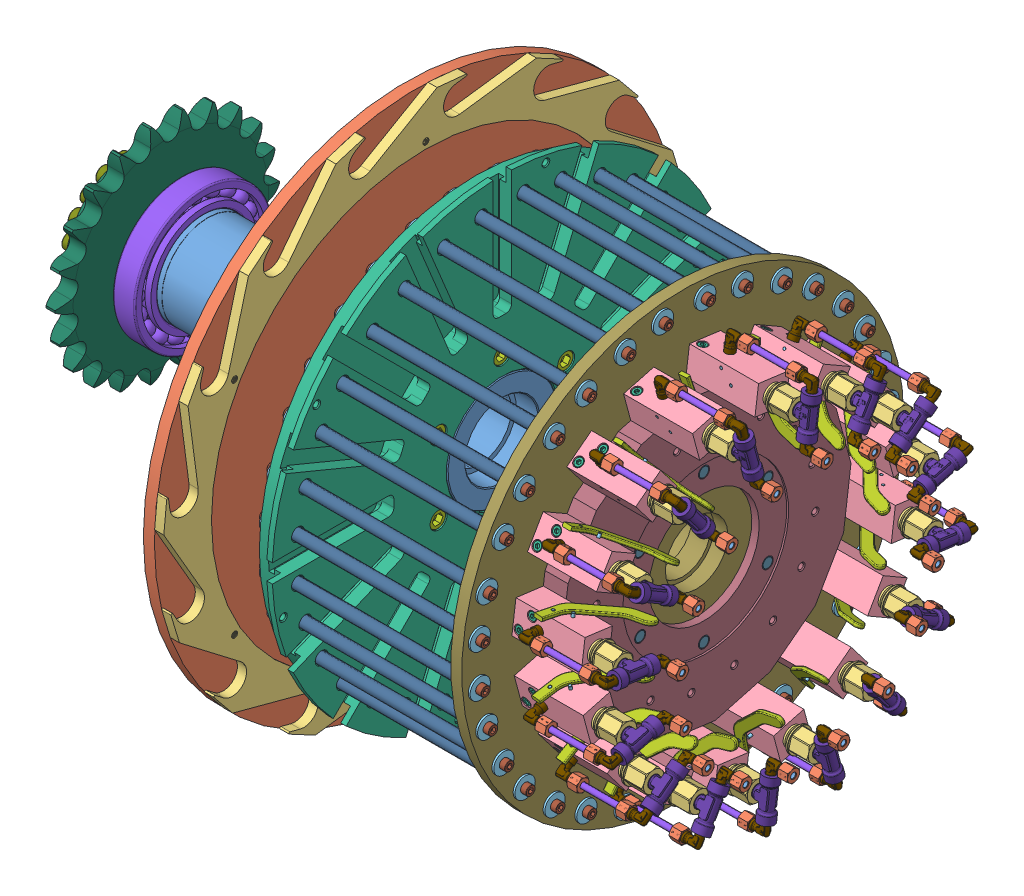
SolidWorks assembly assieme parte rotante, configuration Default. Lengths in mm.
Overall size (749.63 778.63 778.63).
547 component instances, 26 part files, 55 mates.
Components (placement in the parent):
- albero rotazione piatti-1: albero rotazione piatti [Default] at (-23.4119 -16.2033 415) size (415 200 200)
- piatto rotante porta tappi-1: piatto rotante porta tappi [Default] at (15.2184 -16.2033 415) x (0 0 -1) z (1 0 0) size (570 570 20.57)
- disco trasportatore tappi 31-1: disco trasportatore tappi 31 [Default] at (27.2184 -16.2033 415) x (0 -0.5 -0.866025) z (1 0 0) size (570 570 10.42)
- M6 20mm-1: M6 20mm [ISO 4762 M6 x 20 - 20N] at (7.2184 -136.2033 207.1539) x (1 0 0) z (0 -1 0) size (26 10 10)
- rondella m6 22mm-97: rondella m6 22mm [Washer ISO 7094 - 6] at (15.2184 -136.2033 207.1539) x (1 0 0) z (0 0 -1) size (2 22 22)
- rondella m6 22mm-98: rondella m6 22mm [Washer ISO 7094 - 6] at (15.2184 103.7967 207.1539) x (1 0 0) z (0 0.866025 -0.5) size (2 22 22)
- rondella m6 22mm-99: rondella m6 22mm [Washer ISO 7094 - 6] at (15.2184 223.7967 415) x (1 0 0) z (0 0.866025 0.5) size (2 22 22)
- rondella m6 22mm-100: rondella m6 22mm [Washer ISO 7094 - 6] at (15.2184 103.7967 622.8461) size (2 22 22)
- rondella m6 22mm-101: rondella m6 22mm [Washer ISO 7094 - 6] at (15.2184 -136.2033 622.8461) x (1 0 0) z (0 -0.866025 0.5) size (2 22 22)
- rondella m6 22mm-102: rondella m6 22mm [Washer ISO 7094 - 6] at (15.2184 -256.2033 415) x (1 0 0) z (0 -0.866025 -0.5) size (2 22 22)
- M6 20mm-2: M6 20mm [ISO 4762 M6 x 20 - 20N] at (7.2184 103.7967 207.1539) x (1 0 0) z (0 -0.5 -0.866025) size (26 10 10)
- M6 20mm-3: M6 20mm [ISO 4762 M6 x 20 - 20N] at (7.2184 223.7967 415) x (1 0 0) z (0 0.5 -0.866025) size (26 10 10)
- M6 20mm-4: M6 20mm [ISO 4762 M6 x 20 - 20N] at (7.2184 103.7967 622.8461) x (1 0 0) z (0 1 0) size (26 10 10)
- M6 20mm-5: M6 20mm [ISO 4762 M6 x 20 - 20N] at (7.2184 -136.2033 622.8461) x (1 0 0) z (0 0.5 0.866025) size (26 10 10)
- M6 20mm-6: M6 20mm [ISO 4762 M6 x 20 - 20N] at (7.2184 -256.2033 415) x (1 0 0) z (0 -0.5 0.866025) size (26 10 10)
- Disco supporto montaggio e Colonne-1: Disco supporto montaggio e Colonne [Default] at (120.2184 -16.2033 415) x (0 0 -1) z (1 0 0) size (499.6 499.6 29)
- m12 90mm-1: m12 90mm [ISO 4762 M12 x 90 - 90N] at (119.2184 -56.2033 345.718) x (-1 0 0) z (0 -1 0) size (102 18 18)
- m12 90mm-2: m12 90mm [ISO 4762 M12 x 90 - 90N] at (119.2184 -96.2033 415) x (-1 0 0) z (0 -0.5 0.866025) size (102 18 18)
- m12 90mm-3: m12 90mm [ISO 4762 M12 x 90 - 90N] at (119.2184 -56.2033 484.282) x (-1 0 0) z (0 0.5 0.866025) size (102 18 18)
- m12 90mm-4: m12 90mm [ISO 4762 M12 x 90 - 90N] at (119.2184 23.7967 484.282) x (-1 0 0) z (0 1 0) size (102 18 18)
- m12 90mm-5: m12 90mm [ISO 4762 M12 x 90 - 90N] at (119.2184 63.7967 415) x (-1 0 0) z (0 0.5 -0.866025) size (102 18 18)
- m12 90mm-6: m12 90mm [ISO 4762 M12 x 90 - 90N] at (119.2184 23.7967 345.718) x (-1 0 0) z (0 -0.5 -0.866025) size (102 18 18)
- SKF - 6020 - 20,DE,NC,20_68-1: SKF - 6020 - 20,DE,NC,20_68 [SKF - 6020 - 20,DE,NC,20_68] at (-21.7816 -16.2033 415) size (24 150 150)
- SKF - 6020 - 20,DE,NC,20_68-2: SKF - 6020 - 20,DE,NC,20_68 [SKF - 6020 - 20,DE,NC,20_68] at (-216.0316 -16.2033 415) x (1 0 0) z (0 -1 0) size (24 150 150)
- seger 100mm-1: seger 100mm [KS 1336 E - 100] at (-231.0316 -16.2033 415) x (0 0 -1) z (1 0 0) size (107.55 112.98 3)
- asta scorrimento carello-1: asta scorrimento carello [Default] at (203.7184 124.511 241.7588) x (0 0 -1) z (1 0 0) size (12 12 225)
- M6 16mm-7: M6 16mm [ISO 4762 M6 x 16 - 16N] at (83.2184 124.511 241.7588) x (1 0 0) z (0 0 -1) size (22 10 10)
- rondella m6 22mm-1: rondella m6 22mm [Washer ISO 7094 - 6] at (91.2184 124.511 241.7588) x (1 0 0) z (0 0 -1) size (2 22 22)
- M6 16mm-35: M6 16mm [ISO 4762 M6 x 16 - 16N] at (324.2184 124.511 241.7588) x (-1 0 0) z (0 0 1) size (22 10 10)
- rondella m6 22mm-35: rondella m6 22mm [Washer ISO 7094 - 6] at (316.2184 124.511 241.7588) x (-1 0 0) z (0 0 1) size (2 22 22)
- asta scorrimento carello-2: asta scorrimento carello [Default] at (203.7184 157.0379 274.2858) x (0 1 0) z (-1 0 0) size (12 12 225)
- M6 16mm-65: M6 16mm [ISO 4762 M6 x 16 - 16N] at (83.2184 157.0379 274.2858) x (1 0 0) z (0 -1 0) size (22 10 10)
- rondella m6 22mm-65: rondella m6 22mm [Washer ISO 7094 - 6] at (91.2184 157.0379 274.2858) x (1 0 0) z (0 -1 0) size (2 22 22)
- M6 16mm-81: M6 16mm [ISO 4762 M6 x 16 - 16N] at (324.2184 157.0379 274.2858) x (-1 0 0) z (0 1 0) size (22 10 10)
- rondella m6 22mm-81: rondella m6 22mm [Washer ISO 7094 - 6] at (316.2184 157.0379 274.2858) x (-1 0 0) z (0 1 0) size (2 22 22)
- rondella m6 22mm-66: rondella m6 22mm [Washer ISO 7094 - 6] at (91.2184 90.0017 218.7005) x (1 0 0) z (0 -0.92388 0.382683) size (2 22 22)
- rondella m6 22mm-67: rondella m6 22mm [Washer ISO 7094 - 6] at (91.2184 6.7967 193) x (1 0 0) z (0 -0.707107 0.707107) size (2 22 22)
- rondella m6 22mm-68: rondella m6 22mm [Washer ISO 7094 - 6] at (91.2184 -79.9098 201.097) x (1 0 0) z (0 -0.382683 0.92388) size (2 22 22)
- rondella m6 22mm-69: rondella m6 22mm [Washer ISO 7094 - 6] at (91.2184 -156.9175 241.7588) size (2 22 22)
- rondella m6 22mm-70: rondella m6 22mm [Washer ISO 7094 - 6] at (91.2184 -212.5028 308.795) x (1 0 0) z (0 0.382683 0.92388) size (2 22 22)
- rondella m6 22mm-71: rondella m6 22mm [Washer ISO 7094 - 6] at (91.2184 -238.2033 392) x (1 0 0) z (0 0.707107 0.707107) size (2 22 22)
- rondella m6 22mm-72: rondella m6 22mm [Washer ISO 7094 - 6] at (91.2184 -230.1062 478.7065) x (1 0 0) z (0 0.92388 0.382683) size (2 22 22)
- rondella m6 22mm-73: rondella m6 22mm [Washer ISO 7094 - 6] at (91.2184 -189.4444 555.7142) x (1 0 0) z (0 1 0) size (2 22 22)
- rondella m6 22mm-74: rondella m6 22mm [Washer ISO 7094 - 6] at (91.2184 -122.4082 611.2995) x (1 0 0) z (0 0.92388 -0.382683) size (2 22 22)
- rondella m6 22mm-75: rondella m6 22mm [Washer ISO 7094 - 6] at (91.2184 -39.2033 637) x (1 0 0) z (0 0.707107 -0.707107) size (2 22 22)
- rondella m6 22mm-76: rondella m6 22mm [Washer ISO 7094 - 6] at (91.2184 47.5032 628.903) x (1 0 0) z (0 0.382683 -0.92388) size (2 22 22)
- rondella m6 22mm-77: rondella m6 22mm [Washer ISO 7094 - 6] at (91.2184 124.511 588.2412) x (1 0 0) z (0 0 -1) size (2 22 22)
- rondella m6 22mm-78: rondella m6 22mm [Washer ISO 7094 - 6] at (91.2184 180.0963 521.205) x (1 0 0) z (0 -0.382683 -0.92388) size (2 22 22)
- rondella m6 22mm-79: rondella m6 22mm [Washer ISO 7094 - 6] at (91.2184 205.7967 438) x (1 0 0) z (0 -0.707107 -0.707107) size (2 22 22)
- rondella m6 22mm-80: rondella m6 22mm [Washer ISO 7094 - 6] at (91.2184 197.6997 351.2935) x (1 0 0) z (0 -0.92388 -0.382683) size (2 22 22)
- M6 16mm-66: M6 16mm [ISO 4762 M6 x 16 - 16N] at (83.2184 90.0017 218.7005) x (1 0 0) z (0 -0.92388 0.382683) size (22 10 10)
- M6 16mm-67: M6 16mm [ISO 4762 M6 x 16 - 16N] at (83.2184 6.7967 193) x (1 0 0) z (0 -0.707107 0.707107) size (22 10 10)
- M6 16mm-68: M6 16mm [ISO 4762 M6 x 16 - 16N] at (83.2184 -79.9098 201.097) x (1 0 0) z (0 -0.382683 0.92388) size (22 10 10)
- M6 16mm-69: M6 16mm [ISO 4762 M6 x 16 - 16N] at (83.2184 -156.9175 241.7588) size (22 10 10)
- M6 16mm-70: M6 16mm [ISO 4762 M6 x 16 - 16N] at (83.2184 -212.5028 308.795) x (1 0 0) z (0 0.382683 0.92388) size (22 10 10)
- M6 16mm-71: M6 16mm [ISO 4762 M6 x 16 - 16N] at (83.2184 -238.2033 392) x (1 0 0) z (0 0.707107 0.707107) size (22 10 10)
- M6 16mm-72: M6 16mm [ISO 4762 M6 x 16 - 16N] at (83.2184 -230.1062 478.7065) x (1 0 0) z (0 0.92388 0.382683) size (22 10 10)
- M6 16mm-73: M6 16mm [ISO 4762 M6 x 16 - 16N] at (83.2184 -189.4444 555.7142) x (1 0 0) z (0 1 0) size (22 10 10)
- M6 16mm-74: M6 16mm [ISO 4762 M6 x 16 - 16N] at (83.2184 -122.4082 611.2995) x (1 0 0) z (0 0.92388 -0.382683) size (22 10 10)
- M6 16mm-75: M6 16mm [ISO 4762 M6 x 16 - 16N] at (83.2184 -39.2033 637) x (1 0 0) z (0 0.707107 -0.707107) size (22 10 10)
- M6 16mm-76: M6 16mm [ISO 4762 M6 x 16 - 16N] at (83.2184 47.5032 628.903) x (1 0 0) z (0 0.382683 -0.92388) size (22 10 10)
- M6 16mm-77: M6 16mm [ISO 4762 M6 x 16 - 16N] at (83.2184 124.511 588.2412) x (1 0 0) z (0 0 -1) size (22 10 10)
- M6 16mm-78: M6 16mm [ISO 4762 M6 x 16 - 16N] at (83.2184 180.0963 521.205) x (1 0 0) z (0 -0.382683 -0.92388) size (22 10 10)
- M6 16mm-79: M6 16mm [ISO 4762 M6 x 16 - 16N] at (83.2184 205.7967 438) x (1 0 0) z (0 -0.707107 -0.707107) size (22 10 10)
- M6 16mm-80: M6 16mm [ISO 4762 M6 x 16 - 16N] at (83.2184 197.6997 351.2935) x (1 0 0) z (0 -0.92388 -0.382683) size (22 10 10)
- rondella m6 22mm-20: rondella m6 22mm [Washer ISO 7094 - 6] at (91.2184 47.5032 201.097) x (1 0 0) z (0 -0.382683 -0.92388) size (2 22 22)
- rondella m6 22mm-21: rondella m6 22mm [Washer ISO 7094 - 6] at (91.2184 -39.2033 193) x (1 0 0) z (0 -0.707107 -0.707107) size (2 22 22)
- rondella m6 22mm-22: rondella m6 22mm [Washer ISO 7094 - 6] at (91.2184 -122.4082 218.7005) x (1 0 0) z (0 -0.92388 -0.382683) size (2 22 22)
- rondella m6 22mm-23: rondella m6 22mm [Washer ISO 7094 - 6] at (91.2184 -189.4444 274.2858) x (1 0 0) z (0 -1 0) size (2 22 22)
- rondella m6 22mm-24: rondella m6 22mm [Washer ISO 7094 - 6] at (91.2184 -230.1062 351.2935) x (1 0 0) z (0 -0.92388 0.382683) size (2 22 22)
- rondella m6 22mm-25: rondella m6 22mm [Washer ISO 7094 - 6] at (91.2184 -238.2033 438) x (1 0 0) z (0 -0.707107 0.707107) size (2 22 22)
- rondella m6 22mm-26: rondella m6 22mm [Washer ISO 7094 - 6] at (91.2184 -212.5028 521.205) x (1 0 0) z (0 -0.382683 0.92388) size (2 22 22)
- rondella m6 22mm-27: rondella m6 22mm [Washer ISO 7094 - 6] at (91.2184 -156.9175 588.2412) size (2 22 22)
- rondella m6 22mm-28: rondella m6 22mm [Washer ISO 7094 - 6] at (91.2184 -79.9098 628.903) x (1 0 0) z (0 0.382683 0.92388) size (2 22 22)
- rondella m6 22mm-29: rondella m6 22mm [Washer ISO 7094 - 6] at (91.2184 6.7967 637) x (1 0 0) z (0 0.707107 0.707107) size (2 22 22)
- rondella m6 22mm-30: rondella m6 22mm [Washer ISO 7094 - 6] at (91.2184 90.0017 611.2995) x (1 0 0) z (0 0.92388 0.382683) size (2 22 22)
- rondella m6 22mm-31: rondella m6 22mm [Washer ISO 7094 - 6] at (91.2184 157.0379 555.7142) x (1 0 0) z (0 1 0) size (2 22 22)
- rondella m6 22mm-32: rondella m6 22mm [Washer ISO 7094 - 6] at (91.2184 197.6997 478.7065) x (1 0 0) z (0 0.92388 -0.382683) size (2 22 22)
- rondella m6 22mm-33: rondella m6 22mm [Washer ISO 7094 - 6] at (91.2184 205.7967 392) x (1 0 0) z (0 0.707107 -0.707107) size (2 22 22)
- rondella m6 22mm-34: rondella m6 22mm [Washer ISO 7094 - 6] at (91.2184 180.0963 308.795) x (1 0 0) z (0 0.382683 -0.92388) size (2 22 22)
- M6 16mm-20: M6 16mm [ISO 4762 M6 x 16 - 16N] at (83.2184 47.5032 201.097) x (1 0 0) z (0 -0.382683 -0.92388) size (22 10 10)
- M6 16mm-21: M6 16mm [ISO 4762 M6 x 16 - 16N] at (83.2184 -39.2033 193) x (1 0 0) z (0 -0.707107 -0.707107) size (22 10 10)
- M6 16mm-22: M6 16mm [ISO 4762 M6 x 16 - 16N] at (83.2184 -122.4082 218.7005) x (1 0 0) z (0 -0.92388 -0.382683) size (22 10 10)
- M6 16mm-23: M6 16mm [ISO 4762 M6 x 16 - 16N] at (83.2184 -189.4444 274.2858) x (1 0 0) z (0 -1 0) size (22 10 10)
- M6 16mm-24: M6 16mm [ISO 4762 M6 x 16 - 16N] at (83.2184 -230.1062 351.2935) x (1 0 0) z (0 -0.92388 0.382683) size (22 10 10)
- M6 16mm-25: M6 16mm [ISO 4762 M6 x 16 - 16N] at (83.2184 -238.2033 438) x (1 0 0) z (0 -0.707107 0.707107) size (22 10 10)
- M6 16mm-26: M6 16mm [ISO 4762 M6 x 16 - 16N] at (83.2184 -212.5028 521.205) x (1 0 0) z (0 -0.382683 0.92388) size (22 10 10)
- M6 16mm-27: M6 16mm [ISO 4762 M6 x 16 - 16N] at (83.2184 -156.9175 588.2412) size (22 10 10)
- M6 16mm-28: M6 16mm [ISO 4762 M6 x 16 - 16N] at (83.2184 -79.9098 628.903) x (1 0 0) z (0 0.382683 0.92388) size (22 10 10)
- M6 16mm-29: M6 16mm [ISO 4762 M6 x 16 - 16N] at (83.2184 6.7967 637) x (1 0 0) z (0 0.707107 0.707107) size (22 10 10)
- M6 16mm-30: M6 16mm [ISO 4762 M6 x 16 - 16N] at (83.2184 90.0017 611.2995) x (1 0 0) z (0 0.92388 0.382683) size (22 10 10)
- M6 16mm-31: M6 16mm [ISO 4762 M6 x 16 - 16N] at (83.2184 157.0379 555.7142) x (1 0 0) z (0 1 0) size (22 10 10)
- M6 16mm-32: M6 16mm [ISO 4762 M6 x 16 - 16N] at (83.2184 197.6997 478.7065) x (1 0 0) z (0 0.92388 -0.382683) size (22 10 10)
- M6 16mm-33: M6 16mm [ISO 4762 M6 x 16 - 16N] at (83.2184 205.7967 392) x (1 0 0) z (0 0.707107 -0.707107) size (22 10 10)
- M6 16mm-34: M6 16mm [ISO 4762 M6 x 16 - 16N] at (83.2184 180.0963 308.795) x (1 0 0) z (0 0.382683 -0.92388) size (22 10 10)
- M6 16mm-82: M6 16mm [ISO 4762 M6 x 16 - 16N] at (324.2184 90.0017 218.7005) x (-1 0 0) z (0 0.92388 -0.382683) size (22 10 10)
- M6 16mm-83: M6 16mm [ISO 4762 M6 x 16 - 16N] at (324.2184 6.7967 193) x (-1 0 0) z (0 0.707107 -0.707107) size (22 10 10)
- M6 16mm-84: M6 16mm [ISO 4762 M6 x 16 - 16N] at (324.2184 -79.9098 201.097) x (-1 0 0) z (0 0.382683 -0.92388) size (22 10 10)
- M6 16mm-85: M6 16mm [ISO 4762 M6 x 16 - 16N] at (324.2184 -156.9175 241.7588) x (-1 0 0) z (0 0 -1) size (22 10 10)
- M6 16mm-86: M6 16mm [ISO 4762 M6 x 16 - 16N] at (324.2184 -212.5028 308.795) x (-1 0 0) z (0 -0.382683 -0.92388) size (22 10 10)
- M6 16mm-87: M6 16mm [ISO 4762 M6 x 16 - 16N] at (324.2184 -238.2033 392) x (-1 0 0) z (0 -0.707107 -0.707107) size (22 10 10)
- M6 16mm-88: M6 16mm [ISO 4762 M6 x 16 - 16N] at (324.2184 -230.1062 478.7065) x (-1 0 0) z (0 -0.92388 -0.382683) size (22 10 10)
- M6 16mm-89: M6 16mm [ISO 4762 M6 x 16 - 16N] at (324.2184 -189.4444 555.7142) x (-1 0 0) z (0 -1 0) size (22 10 10)
- M6 16mm-90: M6 16mm [ISO 4762 M6 x 16 - 16N] at (324.2184 -122.4082 611.2995) x (-1 0 0) z (0 -0.92388 0.382683) size (22 10 10)
- M6 16mm-91: M6 16mm [ISO 4762 M6 x 16 - 16N] at (324.2184 -39.2033 637) x (-1 0 0) z (0 -0.707107 0.707107) size (22 10 10)
- M6 16mm-92: M6 16mm [ISO 4762 M6 x 16 - 16N] at (324.2184 47.5032 628.903) x (-1 0 0) z (0 -0.382683 0.92388) size (22 10 10)
- M6 16mm-93: M6 16mm [ISO 4762 M6 x 16 - 16N] at (324.2184 124.511 588.2412) x (-1 0 0) z (0 0 1) size (22 10 10)
- M6 16mm-94: M6 16mm [ISO 4762 M6 x 16 - 16N] at (324.2184 180.0963 521.205) x (-1 0 0) z (0 0.382683 0.92388) size (22 10 10)
- M6 16mm-95: M6 16mm [ISO 4762 M6 x 16 - 16N] at (324.2184 205.7967 438) x (-1 0 0) z (0 0.707107 0.707107) size (22 10 10)
- M6 16mm-96: M6 16mm [ISO 4762 M6 x 16 - 16N] at (324.2184 197.6997 351.2935) x (-1 0 0) z (0 0.92388 0.382683) size (22 10 10)
- rondella m6 22mm-82: rondella m6 22mm [Washer ISO 7094 - 6] at (316.2184 90.0017 218.7005) x (-1 0 0) z (0 0.92388 -0.382683) size (2 22 22)
- rondella m6 22mm-83: rondella m6 22mm [Washer ISO 7094 - 6] at (316.2184 6.7967 193) x (-1 0 0) z (0 0.707107 -0.707107) size (2 22 22)
- rondella m6 22mm-84: rondella m6 22mm [Washer ISO 7094 - 6] at (316.2184 -79.9098 201.097) x (-1 0 0) z (0 0.382683 -0.92388) size (2 22 22)
- rondella m6 22mm-85: rondella m6 22mm [Washer ISO 7094 - 6] at (316.2184 -156.9175 241.7588) x (-1 0 0) z (0 0 -1) size (2 22 22)
- rondella m6 22mm-86: rondella m6 22mm [Washer ISO 7094 - 6] at (316.2184 -212.5028 308.795) x (-1 0 0) z (0 -0.382683 -0.92388) size (2 22 22)
- rondella m6 22mm-87: rondella m6 22mm [Washer ISO 7094 - 6] at (316.2184 -238.2033 392) x (-1 0 0) z (0 -0.707107 -0.707107) size (2 22 22)
- rondella m6 22mm-88: rondella m6 22mm [Washer ISO 7094 - 6] at (316.2184 -230.1062 478.7065) x (-1 0 0) z (0 -0.92388 -0.382683) size (2 22 22)
- rondella m6 22mm-89: rondella m6 22mm [Washer ISO 7094 - 6] at (316.2184 -189.4444 555.7142) x (-1 0 0) z (0 -1 0) size (2 22 22)
- rondella m6 22mm-90: rondella m6 22mm [Washer ISO 7094 - 6] at (316.2184 -122.4082 611.2995) x (-1 0 0) z (0 -0.92388 0.382683) size (2 22 22)
- rondella m6 22mm-91: rondella m6 22mm [Washer ISO 7094 - 6] at (316.2184 -39.2033 637) x (-1 0 0) z (0 -0.707107 0.707107) size (2 22 22)
- rondella m6 22mm-92: rondella m6 22mm [Washer ISO 7094 - 6] at (316.2184 47.5032 628.903) x (-1 0 0) z (0 -0.382683 0.92388) size (2 22 22)
- rondella m6 22mm-93: rondella m6 22mm [Washer ISO 7094 - 6] at (316.2184 124.511 588.2412) x (-1 0 0) z (0 0 1) size (2 22 22)
- rondella m6 22mm-94: rondella m6 22mm [Washer ISO 7094 - 6] at (316.2184 180.0963 521.205) x (-1 0 0) z (0 0.382683 0.92388) size (2 22 22)
- rondella m6 22mm-95: rondella m6 22mm [Washer ISO 7094 - 6] at (316.2184 205.7967 438) x (-1 0 0) z (0 0.707107 0.707107) size (2 22 22)
- rondella m6 22mm-96: rondella m6 22mm [Washer ISO 7094 - 6] at (316.2184 197.6997 351.2935) x (-1 0 0) z (0 0.92388 0.382683) size (2 22 22)
- M6 16mm-50: M6 16mm [ISO 4762 M6 x 16 - 16N] at (324.2184 47.5032 201.097) x (-1 0 0) z (0 0.382683 0.92388) size (22 10 10)
- M6 16mm-51: M6 16mm [ISO 4762 M6 x 16 - 16N] at (324.2184 -39.2033 193) x (-1 0 0) z (0 0.707107 0.707107) size (22 10 10)
- M6 16mm-52: M6 16mm [ISO 4762 M6 x 16 - 16N] at (324.2184 -122.4082 218.7005) x (-1 0 0) z (0 0.92388 0.382683) size (22 10 10)
- M6 16mm-53: M6 16mm [ISO 4762 M6 x 16 - 16N] at (324.2184 -189.4444 274.2858) x (-1 0 0) z (0 1 0) size (22 10 10)
- M6 16mm-54: M6 16mm [ISO 4762 M6 x 16 - 16N] at (324.2184 -230.1062 351.2935) x (-1 0 0) z (0 0.92388 -0.382683) size (22 10 10)
- M6 16mm-55: M6 16mm [ISO 4762 M6 x 16 - 16N] at (324.2184 -238.2033 438) x (-1 0 0) z (0 0.707107 -0.707107) size (22 10 10)
- M6 16mm-56: M6 16mm [ISO 4762 M6 x 16 - 16N] at (324.2184 -212.5028 521.205) x (-1 0 0) z (0 0.382683 -0.92388) size (22 10 10)
- M6 16mm-57: M6 16mm [ISO 4762 M6 x 16 - 16N] at (324.2184 -156.9175 588.2412) x (-1 0 0) z (0 0 -1) size (22 10 10)
- M6 16mm-58: M6 16mm [ISO 4762 M6 x 16 - 16N] at (324.2184 -79.9098 628.903) x (-1 0 0) z (0 -0.382683 -0.92388) size (22 10 10)
- M6 16mm-59: M6 16mm [ISO 4762 M6 x 16 - 16N] at (324.2184 6.7967 637) x (-1 0 0) z (0 -0.707107 -0.707107) size (22 10 10)
- M6 16mm-60: M6 16mm [ISO 4762 M6 x 16 - 16N] at (324.2184 90.0017 611.2995) x (-1 0 0) z (0 -0.92388 -0.382683) size (22 10 10)
- M6 16mm-61: M6 16mm [ISO 4762 M6 x 16 - 16N] at (324.2184 157.0379 555.7142) x (-1 0 0) z (0 -1 0) size (22 10 10)
- M6 16mm-62: M6 16mm [ISO 4762 M6 x 16 - 16N] at (324.2184 197.6997 478.7065) x (-1 0 0) z (0 -0.92388 0.382683) size (22 10 10)
- M6 16mm-63: M6 16mm [ISO 4762 M6 x 16 - 16N] at (324.2184 205.7967 392) x (-1 0 0) z (0 -0.707107 0.707107) size (22 10 10)
- M6 16mm-64: M6 16mm [ISO 4762 M6 x 16 - 16N] at (324.2184 180.0963 308.795) x (-1 0 0) z (0 -0.382683 0.92388) size (22 10 10)
- rondella m6 22mm-50: rondella m6 22mm [Washer ISO 7094 - 6] at (316.2184 47.5032 201.097) x (-1 0 0) z (0 0.382683 0.92388) size (2 22 22)
- rondella m6 22mm-51: rondella m6 22mm [Washer ISO 7094 - 6] at (316.2184 -39.2033 193) x (-1 0 0) z (0 0.707107 0.707107) size (2 22 22)
- rondella m6 22mm-52: rondella m6 22mm [Washer ISO 7094 - 6] at (316.2184 -122.4082 218.7005) x (-1 0 0) z (0 0.92388 0.382683) size (2 22 22)
- rondella m6 22mm-53: rondella m6 22mm [Washer ISO 7094 - 6] at (316.2184 -189.4444 274.2858) x (-1 0 0) z (0 1 0) size (2 22 22)
- rondella m6 22mm-54: rondella m6 22mm [Washer ISO 7094 - 6] at (316.2184 -230.1062 351.2935) x (-1 0 0) z (0 0.92388 -0.382683) size (2 22 22)
- rondella m6 22mm-55: rondella m6 22mm [Washer ISO 7094 - 6] at (316.2184 -238.2033 438) x (-1 0 0) z (0 0.707107 -0.707107) size (2 22 22)
- rondella m6 22mm-56: rondella m6 22mm [Washer ISO 7094 - 6] at (316.2184 -212.5028 521.205) x (-1 0 0) z (0 0.382683 -0.92388) size (2 22 22)
- rondella m6 22mm-57: rondella m6 22mm [Washer ISO 7094 - 6] at (316.2184 -156.9175 588.2412) x (-1 0 0) z (0 0 -1) size (2 22 22)
- rondella m6 22mm-58: rondella m6 22mm [Washer ISO 7094 - 6] at (316.2184 -79.9098 628.903) x (-1 0 0) z (0 -0.382683 -0.92388) size (2 22 22)
- rondella m6 22mm-59: rondella m6 22mm [Washer ISO 7094 - 6] at (316.2184 6.7967 637) x (-1 0 0) z (0 -0.707107 -0.707107) size (2 22 22)
- rondella m6 22mm-60: rondella m6 22mm [Washer ISO 7094 - 6] at (316.2184 90.0017 611.2995) x (-1 0 0) z (0 -0.92388 -0.382683) size (2 22 22)
- rondella m6 22mm-61: rondella m6 22mm [Washer ISO 7094 - 6] at (316.2184 157.0379 555.7142) x (-1 0 0) z (0 -1 0) size (2 22 22)
- rondella m6 22mm-62: rondella m6 22mm [Washer ISO 7094 - 6] at (316.2184 197.6997 478.7065) x (-1 0 0) z (0 -0.92388 0.382683) size (2 22 22)
- rondella m6 22mm-63: rondella m6 22mm [Washer ISO 7094 - 6] at (316.2184 205.7967 392) x (-1 0 0) z (0 -0.707107 0.707107) size (2 22 22)
- rondella m6 22mm-64: rondella m6 22mm [Washer ISO 7094 - 6] at (316.2184 180.0963 308.795) x (-1 0 0) z (0 -0.382683 0.92388) size (2 22 22)
- asta scorrimento carello-3: asta scorrimento carello [Default] at (203.7184 47.5032 201.097) x (0 -0.382683 -0.92388) z (1 0 0) size (12 12 225)
- asta scorrimento carello-4: asta scorrimento carello [Default] at (203.7184 -39.2033 193) x (0 -0.707107 -0.707107) z (1 0 0) size (12 12 225)
- asta scorrimento carello-5: asta scorrimento carello [Default] at (203.7184 -122.4082 218.7005) x (0 -0.92388 -0.382683) z (1 0 0) size (12 12 225)
- asta scorrimento carello-6: asta scorrimento carello [Default] at (203.7184 -189.4444 274.2858) x (0 -1 0) z (1 0 0) size (12 12 225)
- asta scorrimento carello-7: asta scorrimento carello [Default] at (203.7184 -230.1062 351.2935) x (0 -0.92388 0.382683) z (1 0 0) size (12 12 225)
- asta scorrimento carello-8: asta scorrimento carello [Default] at (203.7184 -238.2033 438) x (0 -0.707107 0.707107) z (1 0 0) size (12 12 225)
- asta scorrimento carello-9: asta scorrimento carello [Default] at (203.7184 -212.5028 521.205) x (0 -0.382683 0.92388) z (1 0 0) size (12 12 225)
- asta scorrimento carello-10: asta scorrimento carello [Default] at (203.7184 -156.9175 588.2412) x (0 0 1) z (1 0 0) size (12 12 225)
- asta scorrimento carello-11: asta scorrimento carello [Default] at (203.7184 -79.9098 628.903) x (0 0.382683 0.92388) z (1 0 0) size (12 12 225)
- asta scorrimento carello-12: asta scorrimento carello [Default] at (203.7184 6.7967 637) x (0 0.707107 0.707107) z (1 0 0) size (12 12 225)
- asta scorrimento carello-13: asta scorrimento carello [Default] at (203.7184 90.0017 611.2995) x (0 0.92388 0.382683) z (1 0 0) size (12 12 225)
- asta scorrimento carello-14: asta scorrimento carello [Default] at (203.7184 157.0379 555.7142) x (0 1 0) z (1 0 0) size (12 12 225)
- asta scorrimento carello-15: asta scorrimento carello [Default] at (203.7184 197.6997 478.7065) x (0 0.92388 -0.382683) z (1 0 0) size (12 12 225)
- asta scorrimento carello-16: asta scorrimento carello [Default] at (203.7184 205.7967 392) x (0 0.707107 -0.707107) z (1 0 0) size (12 12 225)
- asta scorrimento carello-17: asta scorrimento carello [Default] at (203.7184 180.0963 308.795) x (0 0.382683 -0.92388) z (1 0 0) size (12 12 225)
- asta scorrimento carello-18: asta scorrimento carello [Default] at (203.7184 90.0017 218.7005) x (0 0.92388 -0.382683) z (-1 0 0) size (12 12 225)
- asta scorrimento carello-19: asta scorrimento carello [Default] at (203.7184 6.7967 193) x (0 0.707107 -0.707107) z (-1 0 0) size (12 12 225)
- asta scorrimento carello-20: asta scorrimento carello [Default] at (203.7184 -79.9098 201.097) x (0 0.382683 -0.92388) z (-1 0 0) size (12 12 225)
- asta scorrimento carello-21: asta scorrimento carello [Default] at (203.7184 -156.9175 241.7588) x (0 0 -1) z (-1 0 0) size (12 12 225)
- asta scorrimento carello-22: asta scorrimento carello [Default] at (203.7184 -212.5028 308.795) x (0 -0.382683 -0.92388) z (-1 0 0) size (12 12 225)
- asta scorrimento carello-23: asta scorrimento carello [Default] at (203.7184 -238.2033 392) x (0 -0.707107 -0.707107) z (-1 0 0) size (12 12 225)
- asta scorrimento carello-24: asta scorrimento carello [Default] at (203.7184 -230.1062 478.7065) x (0 -0.92388 -0.382683) z (-1 0 0) size (12 12 225)
- asta scorrimento carello-25: asta scorrimento carello [Default] at (203.7184 -189.4444 555.7142) x (0 -1 0) z (-1 0 0) size (12 12 225)
- asta scorrimento carello-26: asta scorrimento carello [Default] at (203.7184 -122.4082 611.2995) x (0 -0.92388 0.382683) z (-1 0 0) size (12 12 225)
- asta scorrimento carello-27: asta scorrimento carello [Default] at (203.7184 -39.2033 637) x (0 -0.707107 0.707107) z (-1 0 0) size (12 12 225)
- asta scorrimento carello-28: asta scorrimento carello [Default] at (203.7184 47.5032 628.903) x (0 -0.382683 0.92388) z (-1 0 0) size (12 12 225)
- asta scorrimento carello-29: asta scorrimento carello [Default] at (203.7184 124.511 588.2412) x (0 0 1) z (-1 0 0) size (12 12 225)
- asta scorrimento carello-30: asta scorrimento carello [Default] at (203.7184 180.0963 521.205) x (0 0.382683 0.92388) z (-1 0 0) size (12 12 225)
- asta scorrimento carello-31: asta scorrimento carello [Default] at (203.7184 205.7967 438) x (0 0.707107 0.707107) z (-1 0 0) size (12 12 225)
- asta scorrimento carello-32: asta scorrimento carello [Default] at (203.7184 197.6997 351.2935) x (0 0.92388 0.382683) z (-1 0 0) size (12 12 225)
- disco trascinato porta distributore vuoto-2: disco trascinato porta distributore vuoto [Default] at (316.2184 -16.2033 415) x (0 0 1) z (-1 0 0) size (480 480 50)
- Distributore Rotante-1: Distributore Rotante [Default] at (341.2184 -16.2033 415) x (0 -0.5 -0.866025) z (1 0 0) size (310 310 25.54)
- m12 35mm-97: m12 35mm [ISO 4762 M12 x 35 - 35N] at (292.2184 -96.2033 415) size (47 18 18)
- m12 35mm-98: m12 35mm [ISO 4762 M12 x 35 - 35N] at (292.2184 -56.2033 484.282) x (1 0 0) z (0 0.866025 0.5) size (47 18 18)
- m12 35mm-99: m12 35mm [ISO 4762 M12 x 35 - 35N] at (292.2184 23.7967 484.282) x (1 0 0) z (0 0.866025 -0.5) size (47 18 18)
- m12 35mm-100: m12 35mm [ISO 4762 M12 x 35 - 35N] at (292.2184 63.7967 415) x (1 0 0) z (0 0 -1) size (47 18 18)
- m12 35mm-101: m12 35mm [ISO 4762 M12 x 35 - 35N] at (292.2184 23.7967 345.718) x (1 0 0) z (0 -0.866025 -0.5) size (47 18 18)
- m12 35mm-102: m12 35mm [ISO 4762 M12 x 35 - 35N] at (292.2184 -56.2033 345.718) x (1 0 0) z (0 -0.866025 0.5) size (47 18 18)
- pulegia z =50-3: pulegia z =50 [Chain wheel ISO - 22Z 20A-1 --22SB150H40L95.0N] at (-257.7416 -16.2033 415) size (41.88 241.57 243.73)
- calettatore d95-1: calettatore d95 [Default] at (-268.7821 -16.2033 415) size (39.5 135 135)
- AssiemeValvola-1: AssiemeValvola [Default] at (431.5008 -101.2033 267.7757) x (0 0.5 0.866025) z (0 0.866025 -0.5) size (90.26 138.63 38)
  - RaccordoT-1: RaccordoT [Default] at origin size (43 29.75 16.5)
  - Raccordo a L-1: Raccordo a L [Default] at (-30 0 0) x (0 -1 0) z (0 0 -1) size (28.34 25.51 14.01)
    - 1809_06_10_01-1: 1809_06_10_01 [Default] at origin size (22.49 23 10)
    - 1809_06_10_02-1: 1809_06_10_02 [Default] at origin size (6.5 8.5 8.5)
    - 1809_06_10_03-1: 1809_06_10_03 [Default] at origin size (11.02 15.01 14.01)
  - Raccordo a L-2: Raccordo a L [Default] at (30 0 0) x (0 1 0) z (0 0 -1) size (28.34 25.51 14.01)
    - 1809_06_10_01-1: 1809_06_10_01 [Default] at origin size (22.49 23 10)
    - 1809_06_10_02-1: 1809_06_10_02 [Default] at origin size (6.5 8.5 8.5)
    - 1809_06_10_03-1: 1809_06_10_03 [Default] at origin size (11.02 15.01 14.01)
  - TappoChiusura-1: TappoChiusura [Default] at (0 -32 0) x (0 -1 0) z (0 0 1) size (38.28 26.74 26.74)
  - CorpoValvola-1: CorpoValvola [Default] at (-15 -115.2824 0) size (30 75 34)
  - Raccordo a L-3: Raccordo a L [Default] at (-30 -88.2824 0) x (0 1 0) z (0 0 1) size (28.34 25.51 14.01)
    - 1809_06_10_01-1: 1809_06_10_01 [Default] at origin size (22.49 23 10)
    - 1809_06_10_02-1: 1809_06_10_02 [Default] at origin size (6.5 8.5 8.5)
    - 1809_06_10_03-1: 1809_06_10_03 [Default] at origin size (11.02 15.01 14.01)
  - Spina_3x38-1: Spina_3x38 [Default] at (0 -68.2824 -21) x (-1 0 0) z (0 0 1) size (3 3 38)
  - Spina_3x38-2: Spina_3x38 [Default] at (-10 -80.2824 -21) x (0.996193 0.087174 0) z (0 0 1) size (3 3 38)
  - M5 40mm-3: M5 40mm [ISO 4762 M5 x 40 - 40N] at (-14.6 -108.7824 9) size (45 8.5 8.5)
  - M5 40mm-2: M5 40mm [ISO 4762 M5 x 40 - 40N] at (-14.6 -96.7824 -9) size (45 8.5 8.5)
  - LevaValvola-1: LevaValvola [Default] at (-24.507 -86.571 -17) x (0.996193 0.087174 0) z (0 0 1) size (77.55 60.2 4)
  - Tubo-1: Tubo [Default] at (-30 -15.9665 0) x (1 0 0) z (0 -1 0) size (6 6 56.4)
- AssiemeValvola-2: AssiemeValvola [Default] at (431.5008 -151.0733 311.5106) x (0 0.793353 0.608761) z (0 0.608761 -0.793353) size (90.26 138.63 38)
  - RaccordoT-1: RaccordoT [Default] at origin size (43 29.75 16.5)
  - Raccordo a L-1: Raccordo a L [Default] at (-30 0 0) x (0 -1 0) z (0 0 -1) size (28.34 25.51 14.01)
    - 1809_06_10_01-1: 1809_06_10_01 [Default] at origin size (22.49 23 10)
    - 1809_06_10_02-1: 1809_06_10_02 [Default] at origin size (6.5 8.5 8.5)
    - 1809_06_10_03-1: 1809_06_10_03 [Default] at origin size (11.02 15.01 14.01)
  - Raccordo a L-2: Raccordo a L [Default] at (30 0 0) x (0 1 0) z (0 0 -1) size (28.34 25.51 14.01)
    - 1809_06_10_01-1: 1809_06_10_01 [Default] at origin size (22.49 23 10)
    - 1809_06_10_02-1: 1809_06_10_02 [Default] at origin size (6.5 8.5 8.5)
    - 1809_06_10_03-1: 1809_06_10_03 [Default] at origin size (11.02 15.01 14.01)
  - TappoChiusura-1: TappoChiusura [Default] at (0 -32 0) x (0 -1 0) z (0 0 1) size (38.28 26.74 26.74)
  - CorpoValvola-1: CorpoValvola [Default] at (-15 -115.2824 0) size (30 75 34)
  - Raccordo a L-3: Raccordo a L [Default] at (-30 -88.2824 0) x (0 1 0) z (0 0 1) size (28.34 25.51 14.01)
    - 1809_06_10_01-1: 1809_06_10_01 [Default] at origin size (22.49 23 10)
    - 1809_06_10_02-1: 1809_06_10_02 [Default] at origin size (6.5 8.5 8.5)
    - 1809_06_10_03-1: 1809_06_10_03 [Default] at origin size (11.02 15.01 14.01)
  - Spina_3x38-1: Spina_3x38 [Default] at (0 -68.2824 -21) x (-1 0 0) z (0 0 1) size (3 3 38)
  - Spina_3x38-2: Spina_3x38 [Default] at (-10 -80.2824 -21) x (0.996193 0.087174 0) z (0 0 1) size (3 3 38)
  - M5 40mm-3: M5 40mm [ISO 4762 M5 x 40 - 40N] at (-14.6 -108.7824 9) size (45 8.5 8.5)
  - M5 40mm-2: M5 40mm [ISO 4762 M5 x 40 - 40N] at (-14.6 -96.7824 -9) size (45 8.5 8.5)
  - LevaValvola-1: LevaValvola [Default] at (-24.507 -86.571 -17) x (0.996193 0.087174 0) z (0 0 1) size (77.55 60.2 4)
  - Tubo-1: Tubo [Default] at (-30 -15.9665 0) x (1 0 0) z (0 -1 0) size (6 6 56.4)
- AssiemeValvola-3: AssiemeValvola [Default] at (431.5008 -180.4107 371.0008) x (0 0.965926 0.258819) z (0 0.258819 -0.965926) size (90.26 138.63 38)
  - RaccordoT-1: RaccordoT [Default] at origin size (43 29.75 16.5)
  - Raccordo a L-1: Raccordo a L [Default] at (-30 0 0) x (0 -1 0) z (0 0 -1) size (28.34 25.51 14.01)
    - 1809_06_10_01-1: 1809_06_10_01 [Default] at origin size (22.49 23 10)
    - 1809_06_10_02-1: 1809_06_10_02 [Default] at origin size (6.5 8.5 8.5)
    - 1809_06_10_03-1: 1809_06_10_03 [Default] at origin size (11.02 15.01 14.01)
  - Raccordo a L-2: Raccordo a L [Default] at (30 0 0) x (0 1 0) z (0 0 -1) size (28.34 25.51 14.01)
    - 1809_06_10_01-1: 1809_06_10_01 [Default] at origin size (22.49 23 10)
    - 1809_06_10_02-1: 1809_06_10_02 [Default] at origin size (6.5 8.5 8.5)
    - 1809_06_10_03-1: 1809_06_10_03 [Default] at origin size (11.02 15.01 14.01)
  - TappoChiusura-1: TappoChiusura [Default] at (0 -32 0) x (0 -1 0) z (0 0 1) size (38.28 26.74 26.74)
  - CorpoValvola-1: CorpoValvola [Default] at (-15 -115.2824 0) size (30 75 34)
  - Raccordo a L-3: Raccordo a L [Default] at (-30 -88.2824 0) x (0 1 0) z (0 0 1) size (28.34 25.51 14.01)
    - 1809_06_10_01-1: 1809_06_10_01 [Default] at origin size (22.49 23 10)
    - 1809_06_10_02-1: 1809_06_10_02 [Default] at origin size (6.5 8.5 8.5)
    - 1809_06_10_03-1: 1809_06_10_03 [Default] at origin size (11.02 15.01 14.01)
  - Spina_3x38-1: Spina_3x38 [Default] at (0 -68.2824 -21) x (-1 0 0) z (0 0 1) size (3 3 38)
  - Spina_3x38-2: Spina_3x38 [Default] at (-10 -80.2824 -21) x (0.996193 0.087174 0) z (0 0 1) size (3 3 38)
  - M5 40mm-3: M5 40mm [ISO 4762 M5 x 40 - 40N] at (-14.6 -108.7824 9) size (45 8.5 8.5)
  - M5 40mm-2: M5 40mm [ISO 4762 M5 x 40 - 40N] at (-14.6 -96.7824 -9) size (45 8.5 8.5)
  - LevaValvola-1: LevaValvola [Default] at (-24.507 -86.571 -17) x (0.996193 0.087174 0) z (0 0 1) size (77.55 60.2 4)
  - Tubo-1: Tubo [Default] at (-30 -15.9665 0) x (1 0 0) z (0 -1 0) size (6 6 56.4)
- AssiemeValvola-4: AssiemeValvola [Default] at (431.5008 -184.7489 437.1895) x (0 0.991445 -0.130526) z (0 -0.130526 -0.991445) size (90.26 138.63 38)
  - RaccordoT-1: RaccordoT [Default] at origin size (43 29.75 16.5)
  - Raccordo a L-1: Raccordo a L [Default] at (-30 0 0) x (0 -1 0) z (0 0 -1) size (28.34 25.51 14.01)
    - 1809_06_10_01-1: 1809_06_10_01 [Default] at origin size (22.49 23 10)
    - 1809_06_10_02-1: 1809_06_10_02 [Default] at origin size (6.5 8.5 8.5)
    - 1809_06_10_03-1: 1809_06_10_03 [Default] at origin size (11.02 15.01 14.01)
  - Raccordo a L-2: Raccordo a L [Default] at (30 0 0) x (0 1 0) z (0 0 -1) size (28.34 25.51 14.01)
    - 1809_06_10_01-1: 1809_06_10_01 [Default] at origin size (22.49 23 10)
    - 1809_06_10_02-1: 1809_06_10_02 [Default] at origin size (6.5 8.5 8.5)
    - 1809_06_10_03-1: 1809_06_10_03 [Default] at origin size (11.02 15.01 14.01)
  - TappoChiusura-1: TappoChiusura [Default] at (0 -32 0) x (0 -1 0) z (0 0 1) size (38.28 26.74 26.74)
  - CorpoValvola-1: CorpoValvola [Default] at (-15 -115.2824 0) size (30 75 34)
  - Raccordo a L-3: Raccordo a L [Default] at (-30 -88.2824 0) x (0 1 0) z (0 0 1) size (28.34 25.51 14.01)
    - 1809_06_10_01-1: 1809_06_10_01 [Default] at origin size (22.49 23 10)
    - 1809_06_10_02-1: 1809_06_10_02 [Default] at origin size (6.5 8.5 8.5)
    - 1809_06_10_03-1: 1809_06_10_03 [Default] at origin size (11.02 15.01 14.01)
  - Spina_3x38-1: Spina_3x38 [Default] at (0 -68.2824 -21) x (-1 0 0) z (0 0 1) size (3 3 38)
  - Spina_3x38-2: Spina_3x38 [Default] at (-10 -80.2824 -21) x (0.996193 0.087174 0) z (0 0 1) size (3 3 38)
  - M5 40mm-3: M5 40mm [ISO 4762 M5 x 40 - 40N] at (-14.6 -108.7824 9) size (45 8.5 8.5)
  - M5 40mm-2: M5 40mm [ISO 4762 M5 x 40 - 40N] at (-14.6 -96.7824 -9) size (45 8.5 8.5)
  - LevaValvola-1: LevaValvola [Default] at (-24.507 -86.571 -17) x (0.996193 0.087174 0) z (0 0 1) size (77.55 60.2 4)
  - Tubo-1: Tubo [Default] at (-30 -15.9665 0) x (1 0 0) z (0 -1 0) size (6 6 56.4)
- AssiemeValvola-5: AssiemeValvola [Default] at (431.5008 -163.4276 500) x (0 0.866025 -0.5) z (0 -0.5 -0.866025) size (90.26 138.63 38)
  - RaccordoT-1: RaccordoT [Default] at origin size (43 29.75 16.5)
  - Raccordo a L-1: Raccordo a L [Default] at (-30 0 0) x (0 -1 0) z (0 0 -1) size (28.34 25.51 14.01)
    - 1809_06_10_01-1: 1809_06_10_01 [Default] at origin size (22.49 23 10)
    - 1809_06_10_02-1: 1809_06_10_02 [Default] at origin size (6.5 8.5 8.5)
    - 1809_06_10_03-1: 1809_06_10_03 [Default] at origin size (11.02 15.01 14.01)
  - Raccordo a L-2: Raccordo a L [Default] at (30 0 0) x (0 1 0) z (0 0 -1) size (28.34 25.51 14.01)
    - 1809_06_10_01-1: 1809_06_10_01 [Default] at origin size (22.49 23 10)
    - 1809_06_10_02-1: 1809_06_10_02 [Default] at origin size (6.5 8.5 8.5)
    - 1809_06_10_03-1: 1809_06_10_03 [Default] at origin size (11.02 15.01 14.01)
  - TappoChiusura-1: TappoChiusura [Default] at (0 -32 0) x (0 -1 0) z (0 0 1) size (38.28 26.74 26.74)
  - CorpoValvola-1: CorpoValvola [Default] at (-15 -115.2824 0) size (30 75 34)
  - Raccordo a L-3: Raccordo a L [Default] at (-30 -88.2824 0) x (0 1 0) z (0 0 1) size (28.34 25.51 14.01)
    - 1809_06_10_01-1: 1809_06_10_01 [Default] at origin size (22.49 23 10)
    - 1809_06_10_02-1: 1809_06_10_02 [Default] at origin size (6.5 8.5 8.5)
    - 1809_06_10_03-1: 1809_06_10_03 [Default] at origin size (11.02 15.01 14.01)
  - Spina_3x38-1: Spina_3x38 [Default] at (0 -68.2824 -21) x (-1 0 0) z (0 0 1) size (3 3 38)
  - Spina_3x38-2: Spina_3x38 [Default] at (-10 -80.2824 -21) x (0.996193 0.087174 0) z (0 0 1) size (3 3 38)
  - M5 40mm-3: M5 40mm [ISO 4762 M5 x 40 - 40N] at (-14.6 -108.7824 9) size (45 8.5 8.5)
  - M5 40mm-2: M5 40mm [ISO 4762 M5 x 40 - 40N] at (-14.6 -96.7824 -9) size (45 8.5 8.5)
  - LevaValvola-1: LevaValvola [Default] at (-24.507 -86.571 -17) x (0.996193 0.087174 0) z (0 0 1) size (77.55 60.2 4)
  - Tubo-1: Tubo [Default] at (-30 -15.9665 0) x (1 0 0) z (0 -1 0) size (6 6 56.4)
